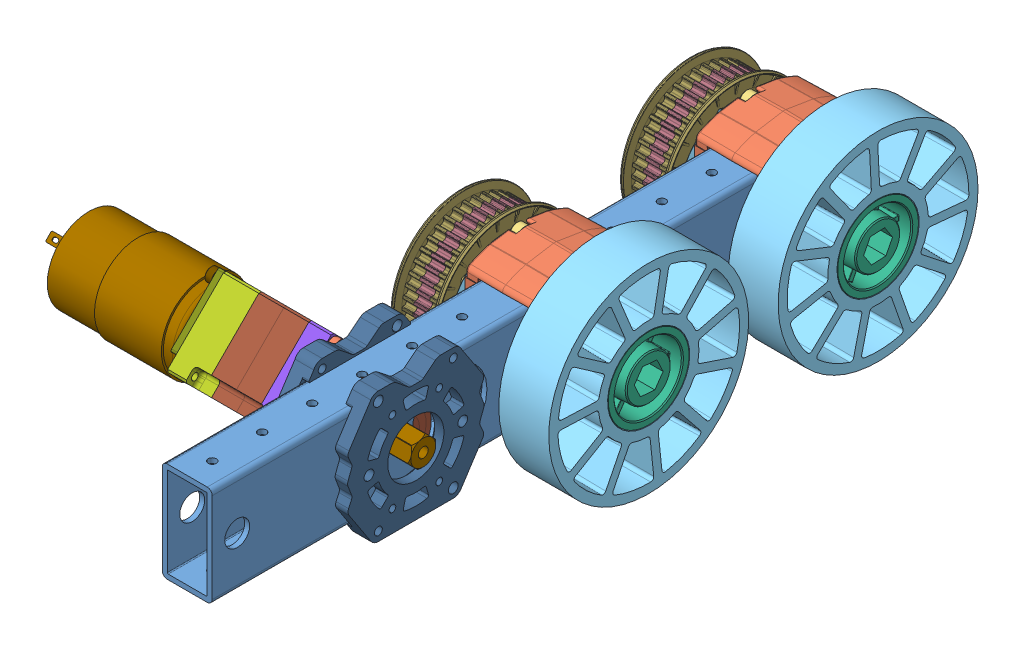
SolidWorks assembly Intake Arm Assembly, configuration Default. Lengths in mm.
Overall size (204.17 141.46 356.77).
77 component instances, 32 part files, 33 mates.
Components (placement in the parent):
- Intake Arm 4-1: Intake Arm 4 [Default] at (110.1918 184.8537 -367.334) size (25.4 50.8 330.2)
- Plastic_Clamping_Bearing_Block_217-4155-1: Plastic_Clamping_Bearing_Block_217-4155 [Default] at (110.2918 184.8537 -636.2941) size (39.75 73.98 53.68)
  - 217-4155-001 Rev6-1: 217-4155-001 Rev6 [Default] at (0 0 714.7682) x (0 0 -1) z (1 0 0) size (53.68 71 22.06)
  - 217-4155-001 Rev6-2: 217-4155-001 Rev6 [Default] at (0 0 714.7682) x (0 0 1) z (-1 0 0) size (53.68 71 22.06)
  - 217-4155-003 Rev1_SSA1032-1375ZB-1: 217-4155-003 Rev1_SSA1032-1375ZB [Default] at (-14.7 29.95 714.7682) x (0 1 0) z (0 0 1) size (7.87 39.75 7.87)
  - 217-4155-003 Rev1_SSA1032-1375ZB-2: 217-4155-003 Rev1_SSA1032-1375ZB [Default] at (-14.7 -29.95 702.0682) x (0 1 0) z (0 0 1) size (7.87 39.75 7.87)
  - 217-4155-003 Rev1_SSA1032-1375ZB-3: 217-4155-003 Rev1_SSA1032-1375ZB [Default] at (-14.7 -29.95 727.4682) x (0 1 0) z (0 0 1) size (7.87 39.75 7.87)
  - 217-4155-002 Rev2_NNY1032-ZC-1: 217-4155-002 Rev2_NNY1032-ZC [Default] at (14.7 29.95 714.7682) x (0 -0.5 -0.866025) z (1 0 0) size (9.39 10.84 4.45)
  - 217-4155-002 Rev2_NNY1032-ZC-2: 217-4155-002 Rev2_NNY1032-ZC [Default] at (14.7 -29.95 702.0682) x (0 -0.5 -0.866025) z (1 0 0) size (9.39 10.84 4.45)
  - 217-4155-002 Rev2_NNY1032-ZC-3: 217-4155-002 Rev2_NNY1032-ZC [Default] at (14.7 -29.95 727.4682) x (0 0.5 -0.866025) z (1 0 0) size (9.39 10.84 4.45)
- am-3480+4IN+500Hex+Bore+Compliant+Wheel-1: am-3480+4IN+500Hex+Bore+Compliant+Wheel [Default] at (139.2648 180.2188 62.0646) x (0 0.049955 -0.998751) z (1 0 0) size (101.6 101.6 25.74)
  - 4IN Compliant Wheel FINAL Overmold-1: 4IN Compliant Wheel FINAL Overmold [Default] at (-16.2374 3.8509 18.652) size (101.6 101.6 25.74)
  - 2in Wheel Intergrated 0500 HEX Hub-1: 2in Wheel Intergrated 0500 HEX Hub [Default] at (-16.2374 3.8509 5.952) x (-1 0 0) z (0 0 -1) size (41.91 41.91 25.4)
- Plastic_Clamping_Bearing_Block_217-4155-2: Plastic_Clamping_Bearing_Block_217-4155 [Default] at (110.0918 184.8537 -519.8761) size (39.75 73.98 53.68)
  - 217-4155-001 Rev6-1: 217-4155-001 Rev6 [Default] at (0 0 714.7682) x (0 0 -1) z (1 0 0) size (53.68 71 22.06)
  - 217-4155-001 Rev6-2: 217-4155-001 Rev6 [Default] at (0 0 714.7682) x (0 0 1) z (-1 0 0) size (53.68 71 22.06)
  - 217-4155-003 Rev1_SSA1032-1375ZB-1: 217-4155-003 Rev1_SSA1032-1375ZB [Default] at (-14.7 29.95 714.7682) x (0 1 0) z (0 0 1) size (7.87 39.75 7.87)
  - 217-4155-003 Rev1_SSA1032-1375ZB-2: 217-4155-003 Rev1_SSA1032-1375ZB [Default] at (-14.7 -29.95 702.0682) x (0 1 0) z (0 0 1) size (7.87 39.75 7.87)
  - 217-4155-003 Rev1_SSA1032-1375ZB-3: 217-4155-003 Rev1_SSA1032-1375ZB [Default] at (-14.7 -29.95 727.4682) x (0 1 0) z (0 0 1) size (7.87 39.75 7.87)
  - 217-4155-002 Rev2_NNY1032-ZC-1: 217-4155-002 Rev2_NNY1032-ZC [Default] at (14.7 29.95 714.7682) x (0 -0.5 -0.866025) z (1 0 0) size (9.39 10.84 4.45)
  - 217-4155-002 Rev2_NNY1032-ZC-2: 217-4155-002 Rev2_NNY1032-ZC [Default] at (14.7 -29.95 702.0682) x (0 -0.5 -0.866025) z (1 0 0) size (9.39 10.84 4.45)
  - 217-4155-002 Rev2_NNY1032-ZC-3: 217-4155-002 Rev2_NNY1032-ZC [Default] at (14.7 -29.95 727.4682) x (0 0.5 -0.866025) z (1 0 0) size (9.39 10.84 4.45)
- 217-2 Stage Versaplanetary STEP-1: 217-2 Stage Versaplanetary STEP [Default] at (39.6168 183.2027 284.7989) x (0 0.707107 -0.707107) z (-1 0 0) size (44.3 44.3 179.1)
  - 217-2625-001 Rev1-1: 217-2625-001 Rev1 [Default] at origin size (42 42 18)
  - 217-2625-002 Rev1-1: 217-2625-002 Rev1 [Default] at (0 0 -29.4) size (42 42 17.13)
  - 217-2625-003 Rev1-1: 217-2625-003 Rev1 [Default] at (0 0 -43.6478) x (1 0 0) z (0 0 -1) size (17 17 64.12)
  - 217-2625-009 Rev1-1: 217-2625-009 Rev1 [Default] at (0 0 -3.48) x (0 -1 0) z (0 0 -1) size (18 18 13)
  - 217-2816-001 Rev1-1: 217-2816-001 Rev1 [Default] at (0 0 -16.85) x (1 0 0) z (0 0 -1) size (42 42 14.5)
  - 217-2625-007 Rev1_Sun_Driver01-1: 217-2625-007 Rev1_Sun_Driver01 [Default] at (0 0 -11.767) x (0.055822 0.998441 0) z (0 0 1) size (14.49 14.49 12.72)
  - 217-2625-100-1: 217-2625-100 [Default] at (0 0 -18.467) x (0 1 0) z (0 0 1) size (39.26 38.9 12.7)
    - 217-2625-008 Rev1-1: 217-2625-008 Rev1 [Default] at origin size (34.7 34.7 4.7)
    - 217-2625-010 Rev1-1: 217-2625-010 Rev1 [Default] at (0 10.193 3.65) x (0.999813 0.019336 0) z (0 0 1) size (4 4 12)
    - 217-2625-010 Rev1-2: 217-2625-010 Rev1 [Default] at (8.691 -5.3258 3.65) size (4 4 12)
    - 217-2625-010 Rev1-3: 217-2625-010 Rev1 [Default] at (-8.691 -5.3258 3.65) size (4 4 12)
    - 217-2625-005 Rev1_Planet_Revolving_Follower01-1: 217-2625-005 Rev1_Planet_Revolving_Follower01 [Default] at (8.691 -5.3258 6.35) x (0.932816 0.360354 0) z (0 0 1) size (16.91 16.92 8)
    - 217-2625-005 Rev1_Planet_Revolving_Follower01-2: 217-2625-005 Rev1_Planet_Revolving_Follower01 [Default] at (-8.691 -5.3258 6.35) x (-0.932788 -0.360426 0) z (0 0 1) size (16.91 16.92 8)
    - 217-2625-005 Rev1_Planet_Revolving_Follower01-3: 217-2625-005 Rev1_Planet_Revolving_Follower01 [Default] at (0 10.193 6.35) x (0.893583 0.448898 0) z (0 0 1) size (16.91 16.92 8)
  - 217-2822-003 Rev4-1: 217-2822-003 Rev4 [Default] at (0 0 9) x (0 1 0) z (0 0 1) size (42 42 4.8)
  - 217-2625-011 Rev1-1: 217-2625-011 Rev1 [Default] at (0 0 1.37) x (1 0 0) z (0 -1 0) size (8.01 7.5 7.94)
  - SSA_SSA0832-0500ZC-1: SSA_SSA0832-0500ZC [Default] at (17.5 -17.5 10.5) x (0.189399 -0.9819 0) z (-0.9819 -0.189399 0) size (6.73 16.76 6.73)
  - 217-2742-1: 217-2742 [Default] at (0 0 -43.1002) x (0 0 1) z (-1 0 0) size (7 28 28)
  - 217-2742-2: 217-2742 [Default] at (0 0 -51.4002) x (0 0 1) z (-0.997393 0.072165 0) size (7 28 28)
  - SSA_SSA0832-1750ZC-1: SSA_SSA0832-1750ZC [Default] at (17.5 -17.5 -47.261) x (1 0 0) z (0 1 0) size (6.73 48.51 6.73)
  - SSA_SSA0832-1750ZC-2: SSA_SSA0832-1750ZC [Default] at (-17.5 17.5 -47.261) x (1 0 0) z (0 1 0) size (6.73 48.51 6.73)
  - 217-2625-018 Rev1_98541A410-1: 217-2625-018 Rev1_98541A410 [Default] at (0 0 -35.4954) x (0 0 -1) z (0.980859 -0.194721 0) size (1 19.6 17.4)
  - 217-2625-017 Rev1_9714K61-1: 217-2625-017 Rev1_9714K61 [Default] at (0 0 -44.1002) x (-0.695225 0.718792 0) z (-0.718792 -0.695225 0) size (28.51 4.98 30.18)
  - PINL-M020-006-S-1: PINL-M020-006-S [Default] at (-18.5 13.6657 -9.5) x (0 0 -1) z (1 0 0) size (6 2 2)
  - PINL-M020-006-S-2: PINL-M020-006-S [Default] at (-18.5 13.6657 -22.2) x (0 0 -1) z (0.23951 -0.970894 0) size (6 2 2)
  - 217-2816-001 Rev1-2: 217-2816-001 Rev1 [Default] at (0 0 -29.55) x (1 0 0) z (0 0 -1) size (42 42 14.5)
  - 217-3106-000 Rev2_NO SUN-1: 217-3106-000 Rev2_NO SUN [Default] at (0 0 -31.5454) size (40.34 37.58 17.71)
    - 217-3106-002 Rev1_Planet_Revolving_Follower01-1: 217-3106-002 Rev1_Planet_Revolving_Follower01 [Default] at (0 10.2965 6.35) x (0.979503 -0.20143 0) z (0 0 1) size (16.8 16.83 8)
    - 217-3106-003 Rev1-1: 217-3106-003 Rev1 [Default] at origin size (34.7 34.7 4.7)
    - 217-3106-001 Rev1_Sun_Driver01-1: 217-3106-001 Rev1_Sun_Driver01 [Default] at (0 0 9.0125) x (1 0 0) z (0 0 -1) size (14.56 14.56 12.7)
    - 217-3106-002 Rev1_Planet_Revolving_Follower01-2: 217-3106-002 Rev1_Planet_Revolving_Follower01 [Default] at (8.917 -5.1482 6.35) x (-0.664195 -0.74756 0) z (0 0 1) size (16.8 16.83 8)
    - 217-3106-002 Rev1_Planet_Revolving_Follower01-3: 217-3106-002 Rev1_Planet_Revolving_Follower01 [Default] at (-8.917 -5.1482 6.35) x (-0.315308 0.948989 0) z (0 0 1) size (16.8 16.83 8)
    - 217-2625-010 Rev1-1: 217-2625-010 Rev1 [Default] at (8.917 -5.1482 3.65) x (0.999617 0.027658 0) z (0 0 1) size (4 4 12)
    - 217-2625-010 Rev1-2: 217-2625-010 Rev1 [Default] at (-8.917 -5.1482 3.65) x (-0.475856 -0.879523 0) z (0 0 1) size (4 4 12)
    - 217-2625-010 Rev1-3: 217-2625-010 Rev1 [Default] at (0 10.2965 3.65) x (-0.523761 0.851865 0) z (0 0 1) size (4 4 12)
  - 775 pro-1: 775 pro [Default] at (0 0 10.5) x (0 0 1) z (-1 0 0) size (88 44.3 44.3)
- 217-3432-STEP-v2-1: 217-3432-STEP-v2 [Default] at (95.9043 184.7902 284.7989) x (0 0 1) z (-1 0 0) size (69.4 66.32 9.53)
- 217-3432-STEP-v2-2: 217-3432-STEP-v2 [Default] at (124.4793 184.7902 284.7989) x (0 0 -1) z (1 0 0) size (69.4 66.32 9.53)
- 18t x 15mm Wide Aluminum Pulley (HTD 5mm, 0.5 inch Hex)-1: 18t x 15mm Wide Aluminum Pulley (HTD 5mm, 0.5 inch Hex) [Default] at (110.0793 183.2027 284.7989) x (0 0.170151 -0.985418) z (1 0 0) size (32 32 22)
- am-3480+4IN+500Hex+Bore+Compliant+Wheel-2: am-3480+4IN+500Hex+Bore+Compliant+Wheel [Default] at (139.0648 194.3676 182.4436) x (0 0.82015 -0.572148) z (1 0 0) size (101.6 101.6 25.74)
  - 4IN Compliant Wheel FINAL Overmold-1: 4IN Compliant Wheel FINAL Overmold [Default] at (-16.2374 3.8509 18.652) size (101.6 101.6 25.74)
  - 2in Wheel Intergrated 0500 HEX Hub-1: 2in Wheel Intergrated 0500 HEX Hub [Default] at (-16.2374 3.8509 5.952) x (-1 0 0) z (0 0 -1) size (41.91 41.91 25.4)
- 42t x 18mm Wide VersaPulley Kit (HTD 5mm, VersaKeys)-1: 42t x 18mm Wide VersaPulley Kit (HTD 5mm, VersaKeys) [Default] at (83.1043 183.2537 194.8921) x (0 -0.173155 -0.984895) z (1 0 0) size (73 73 23.01)
  - 217-3199-001 Rev4-1: 217-3199-001 Rev4 [Default] at origin size (73 73 11.51)
  - 217-3199-001 Rev4-2: 217-3199-001 Rev4 [Default] at (0 0 -17.825) x (-1 0 0) z (0 0 -1) size (73 73 11.51)
  - 217-3199-002 Rev3-1: 217-3199-002 Rev3 [Default] at (0 0 -5.5) x (-1 0 0) z (0 0 1) size (65.74 65.61 14)
- 1_2_Hex_Bore_Plastic_VersaHub_217-4009-1: 1_2_Hex_Bore_Plastic_VersaHub_217-4009 [Default] at (62.1043 183.2537 194.8921) x (0 -0.008287 -0.999966) z (1 0 0) size (54.75 55.87 12.7)
- 1_2_Hex_Bore_Plastic_VersaHub_217-4009-2: 1_2_Hex_Bore_Plastic_VersaHub_217-4009 [Default] at (86.2793 183.2537 194.8921) x (0 0.921028 0.389495) z (-1 0 0) size (54.75 55.87 12.7)
- 1_2_Hex_Bore_Plastic_VersaHub_217-4009-3: 1_2_Hex_Bore_Plastic_VersaHub_217-4009 [Default] at (62.3043 183.2537 78.4741) x (0 -0.008287 -0.999966) z (1 0 0) size (54.75 55.87 12.7)
- 1_2_Hex_Bore_Plastic_VersaHub_217-4009-4: 1_2_Hex_Bore_Plastic_VersaHub_217-4009 [Default] at (86.4793 183.2537 78.4741) x (0 0.921028 0.389495) z (-1 0 0) size (54.75 55.87 12.7)
- 42t x 18mm Wide VersaPulley Kit (HTD 5mm, VersaKeys)-2: 42t x 18mm Wide VersaPulley Kit (HTD 5mm, VersaKeys) [Default] at (83.3043 183.2537 78.4741) x (0 0.269121 -0.963106) z (1 0 0) size (73 73 23.01)
  - 217-3199-001 Rev4-1: 217-3199-001 Rev4 [Default] at origin size (73 73 11.51)
  - 217-3199-001 Rev4-2: 217-3199-001 Rev4 [Default] at (0 0 -17.825) x (-1 0 0) z (0 0 -1) size (73 73 11.51)
  - 217-3199-002 Rev3-1: 217-3199-002 Rev3 [Default] at (0 0 -5.5) x (-1 0 0) z (0 0 1) size (65.74 65.61 14)
Mates (geometry in assembly coordinates):
- Coincident1: coincident anti-aligned: plane of Intake Arm 4-1 through (100.0318 159.4537 381.966) normal (0 -1 0); plane of Plastic_Clamping_Bearing_Block_217-4155-1/217-4155-001 Rev6-2 through (97.6918 159.4537 118.4741) normal (0 1 0)
- Coincident2: coincident anti-aligned: plane of Intake Arm 4-1 through (122.8918 161.9937 381.966) normal (1 0 0); plane of Plastic_Clamping_Bearing_Block_217-4155-1/217-4155-001 Rev6-1 through (122.8918 184.8537 78.4741) normal (-1 0 0)
- Coincident3: coincident aligned: plane of Intake Arm 4-1 through (110.1918 184.8537 51.766) normal (0 0 -1); plane of Plastic_Clamping_Bearing_Block_217-4155-1/217-4155-001 Rev6-2 through (97.6918 207.8537 51.766) normal (0 0 -1)
- Concentric1: concentric anti-aligned: circle of Plastic_Clamping_Bearing_Block_217-4155-1/217-4155-001 Rev6-2; circle of am-3480+4IN+500Hex+Bore+Compliant+Wheel-1/4IN Compliant Wheel FINAL Overmold-1
- Distance1: distance = 3.175 mm anti-aligned: plane of am-3480+4IN+500Hex+Bore+Compliant+Wheel-1/2in Wheel Intergrated 0500 HEX Hub-1 through (132.5168 185.7905 78.601) normal (-1 0 0); plane of Plastic_Clamping_Bearing_Block_217-4155-1/217-4155-001 Rev6-1 through (129.3418 213.6037 64.4741) normal (1 0 0)
- Coincident4: coincident anti-aligned: plane of Intake Arm 4-1 through (97.4918 161.9937 381.966) normal (-1 0 0); plane of Plastic_Clamping_Bearing_Block_217-4155-2/217-4155-001 Rev6-2 through (97.4918 184.8537 194.8921) normal (1 0 0)
- Coincident5: coincident anti-aligned: plane of Intake Arm 4-1 through (100.0318 159.4537 381.966) normal (0 -1 0); plane of Plastic_Clamping_Bearing_Block_217-4155-2/217-4155-001 Rev6-1 through (122.6918 159.4537 154.8921) normal (0 1 0)
- Coincident7: coincident anti-aligned: plane of 217-2 Stage Versaplanetary STEP-1/217-2625-002 Rev1-1 through (91.1418 153.5042 284.7989) normal (1 0 0); plane of 217-3432-STEP-v2-1 through (91.1418 184.7902 284.7989) normal (-1 0 0)
- Concentric2: concentric aligned: circle of 217-2 Stage Versaplanetary STEP-1/217-2625-002 Rev1-1; cylinder of 217-3432-STEP-v2-1 through (91.1418 183.2027 284.7989) axis (1 0 0) radius 14.2748
- Angle1: planar angle = 0.785398 rad aligned: plane of 217-3432-STEP-v2-1 through (91.1418 151.6305 284.7989) normal (0 -1 0); plane of 217-2 Stage Versaplanetary STEP-1/217-2625-002 Rev1-1 through (91.1418 183.2027 255.1004) normal (0 -0.707107 -0.707107)
- Coincident8: coincident aligned: plane of 217-3432-STEP-v2-1 through (91.1418 151.6305 284.7989) normal (0 -1 0); plane of 217-3432-STEP-v2-2 through (129.2418 151.6305 284.7989) normal (0 -1 0)
- Concentric3: concentric anti-aligned: cylinder of 217-3432-STEP-v2-1 through (91.1418 183.2027 284.7989) axis (1 0 0) radius 14.2748; cylinder of 217-3432-STEP-v2-2 through (129.2418 183.2027 284.7989) axis (-1 0 0) radius 14.2748
- Distance4: distance = 25.4 mm anti-aligned: plane of 217-3432-STEP-v2-1 through (97.4918 184.7902 284.7989) normal (1 0 0); plane of 217-3432-STEP-v2-2 through (122.8918 184.7902 284.7989) normal (-1 0 0)
- Concentric4: concentric anti-aligned: cylinder of 217-3432-STEP-v2-1 through (91.1418 183.2027 284.7989) axis (1 0 0) radius 14.2748; cylinder of 18t x 15mm Wide Aluminum Pulley (HTD 5mm, 0.5 inch Hex)-1 through (110.0793 183.2027 284.7989) axis (-1 0 0) radius 16
- Distance5: distance = 1.5875 mm anti-aligned: plane of 18t x 15mm Wide Aluminum Pulley (HTD 5mm, 0.5 inch Hex)-1 through (99.0793 183.2027 284.7989) normal (-1 0 0); plane of 217-3432-STEP-v2-1 through (97.4918 184.7902 284.7989) normal (1 0 0)
- Coincident9: coincident anti-aligned: plane of Intake Arm 4-1 through (97.4918 161.9937 381.966) normal (-1 0 0); plane of 217-3432-STEP-v2-1 through (97.4918 184.7902 284.7989) normal (1 0 0)
- Coincident10: coincident anti-aligned: plane of Intake Arm 4-1 through (100.0318 210.2537 381.966) normal (0 1 0); plane of 217-3432-STEP-v2-1 through (97.4918 210.2537 360.9989) normal (0 -1 0)
- Distance6: distance = 177.8 mm: cylinder of Plastic_Clamping_Bearing_Block_217-4155-1/217-4155-001 Rev6-1 through (129.3418 183.2537 78.4741) axis (-1 0 0) radius 14.25; cylinder of 217-3432-STEP-v2-2 through (129.2418 183.2027 284.7989) axis (-1 0 0) radius 14.2748
- Concentric5: concentric aligned: cylinder of Plastic_Clamping_Bearing_Block_217-4155-2/217-4155-001 Rev6-1 through (129.1418 183.2537 194.8921) axis (-1 0 0) radius 14.25; cylinder of am-3480+4IN+500Hex+Bore+Compliant+Wheel-2/4IN Compliant Wheel FINAL Overmold-1 through (187.513 183.2537 194.8921) axis (-1 0 0) radius 50.8
- Distance7: distance = 3.175 mm anti-aligned: plane of Plastic_Clamping_Bearing_Block_217-4155-2/217-4155-001 Rev6-1 through (129.1418 213.6037 180.8921) normal (1 0 0); plane of am-3480+4IN+500Hex+Bore+Compliant+Wheel-2/2in Wheel Intergrated 0500 HEX Hub-1 through (132.3168 184.707 196.9753) normal (-1 0 0)
- Concentric6: concentric anti-aligned: cylinder of 42t x 18mm Wide VersaPulley Kit (HTD 5mm, VersaKeys)-1/217-3199-001 Rev4-2 through (63.6918 183.2537 194.8921) axis (1 0 0) radius 14.3; cylinder of 1_2_Hex_Bore_Plastic_VersaHub_217-4009-1 through (73.2168 183.2537 194.8921) axis (-1 0 0) radius 14.3002
- Coincident11: coincident anti-aligned: plane of 42t x 18mm Wide VersaPulley Kit (HTD 5mm, VersaKeys)-1/217-3199-001 Rev4-2 through (63.6918 183.2537 194.8921) normal (-1 0 0); plane of 1_2_Hex_Bore_Plastic_VersaHub_217-4009-1 through (63.6918 183.2537 194.8921) normal (1 0 0)
- Concentric7: concentric anti-aligned: cylinder of Plastic_Clamping_Bearing_Block_217-4155-2/217-4155-001 Rev6-2 through (91.0418 183.2537 194.8921) axis (1 0 0) radius 14.25; cylinder of 42t x 18mm Wide VersaPulley Kit (HTD 5mm, VersaKeys)-1/217-3199-001 Rev4-1 through (84.6918 183.2537 194.8921) axis (-1 0 0) radius 14.3
- Concentric8: concentric aligned: cylinder of 42t x 18mm Wide VersaPulley Kit (HTD 5mm, VersaKeys)-1/217-3199-001 Rev4-1 through (84.6918 183.2537 194.8921) axis (-1 0 0) radius 14.3; cone of 1_2_Hex_Bore_Plastic_VersaHub_217-4009-2 through (78.3418 183.2537 194.8921) axis (-1 0 0)
- Coincident12: coincident anti-aligned: plane of 42t x 18mm Wide VersaPulley Kit (HTD 5mm, VersaKeys)-1/217-3199-001 Rev4-1 through (84.6918 183.2537 194.8921) normal (1 0 0); plane of 1_2_Hex_Bore_Plastic_VersaHub_217-4009-2 through (84.6918 183.2537 194.8921) normal (-1 0 0)
- Concentric9: concentric aligned: cone of 1_2_Hex_Bore_Plastic_VersaHub_217-4009-4 through (78.5418 183.2537 78.4741) axis (-1 0 0); cylinder of 42t x 18mm Wide VersaPulley Kit (HTD 5mm, VersaKeys)-2/217-3199-001 Rev4-1 through (84.8918 183.2537 78.4741) axis (-1 0 0) radius 14.3
- Coincident13: coincident anti-aligned: plane of 1_2_Hex_Bore_Plastic_VersaHub_217-4009-3 through (63.8918 183.2537 78.4741) normal (1 0 0); plane of 42t x 18mm Wide VersaPulley Kit (HTD 5mm, VersaKeys)-2/217-3199-001 Rev4-2 through (63.8918 183.2537 78.4741) normal (-1 0 0)
- Coincident14: coincident anti-aligned: plane of 1_2_Hex_Bore_Plastic_VersaHub_217-4009-4 through (84.8918 183.2537 78.4741) normal (-1 0 0); plane of 42t x 18mm Wide VersaPulley Kit (HTD 5mm, VersaKeys)-2/217-3199-001 Rev4-1 through (84.8918 183.2537 78.4741) normal (1 0 0)
- Concentric10: concentric anti-aligned: cylinder of 1_2_Hex_Bore_Plastic_VersaHub_217-4009-3 through (73.4168 183.2537 78.4741) axis (-1 0 0) radius 14.3002; cylinder of 42t x 18mm Wide VersaPulley Kit (HTD 5mm, VersaKeys)-2/217-3199-001 Rev4-2 through (63.8918 183.2537 78.4741) axis (1 0 0) radius 14.3
- Concentric11: concentric aligned: cylinder of Plastic_Clamping_Bearing_Block_217-4155-2/217-4155-001 Rev6-2 through (91.0418 183.2537 194.8921) axis (1 0 0) radius 14.25; circle of 42t x 18mm Wide VersaPulley Kit (HTD 5mm, VersaKeys)-1/217-3199-001 Rev4-1
- Distance8: distance = 3.175 mm anti-aligned: plane of Plastic_Clamping_Bearing_Block_217-4155-2/217-4155-001 Rev6-2 through (91.0418 213.6037 208.8921) normal (-1 0 0); plane of 1_2_Hex_Bore_Plastic_VersaHub_217-4009-2 through (87.8668 183.2537 194.8921) normal (1 0 0)
- Concentric12: concentric aligned: cylinder of Plastic_Clamping_Bearing_Block_217-4155-1/217-4155-001 Rev6-2 through (91.2418 183.2537 78.4741) axis (1 0 0) radius 14.25; circle of 42t x 18mm Wide VersaPulley Kit (HTD 5mm, VersaKeys)-2/217-3199-001 Rev4-1
- Distance9: distance = 3.175 mm anti-aligned: plane of Plastic_Clamping_Bearing_Block_217-4155-1/217-4155-001 Rev6-2 through (91.2418 213.6037 92.4741) normal (-1 0 0); plane of 1_2_Hex_Bore_Plastic_VersaHub_217-4009-4 through (88.0668 183.2537 78.4741) normal (1 0 0)
